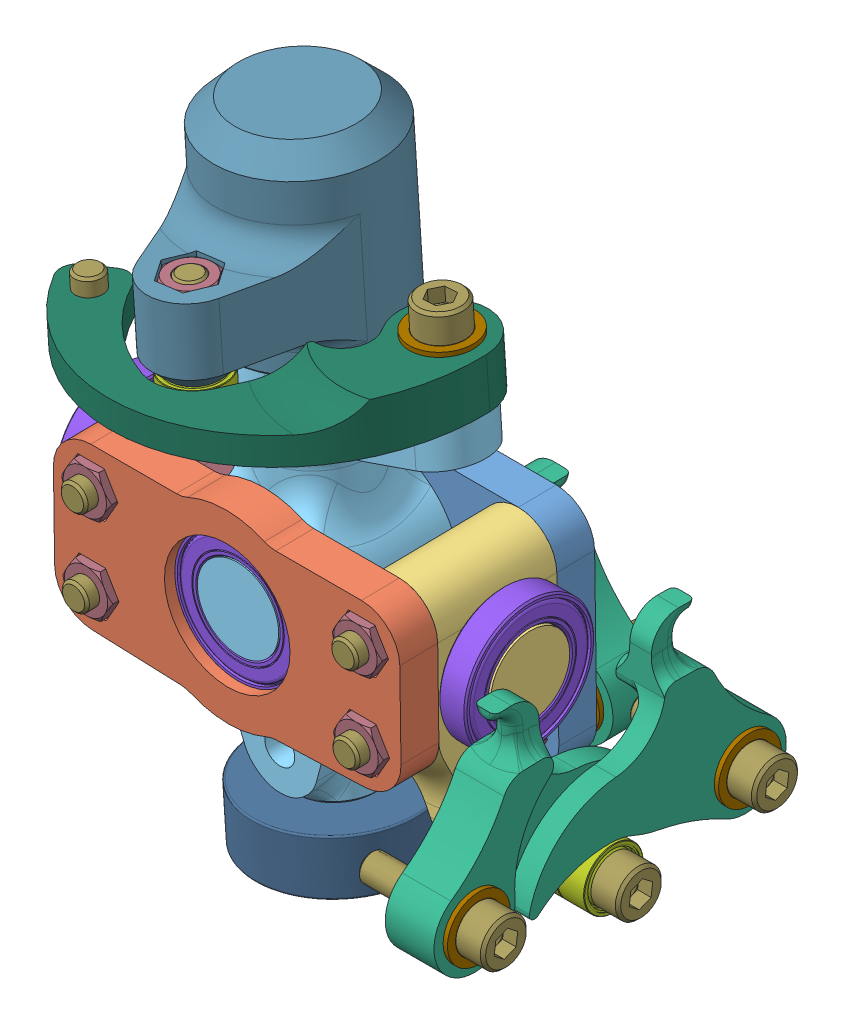
SolidWorks assembly Axis Assembly, configuration Default. Lengths in mm.
58 component instances, 15 part files, 133 mates.
Components (placement in the parent):
- gimbal_core_bearing_carrier_non_pot_side-1: gimbal_core_bearing_carrier_non_pot_side [Default] at (-18 0.2008 -14.4986) x (-1 0 0) z (0 0.013848 -0.999904) size (64 44 7.5)
- gimbal_core_bearing_carrier_pot_side-1: gimbal_core_bearing_carrier_pot_side [Default] at (-18 -0.2008 14.4986) x (1 0 0) z (0 -0.013848 0.999904) size (64 34.5 7)
- gimbal_core_non_pot_side-1: gimbal_core_non_pot_side [Default] x (0 0.013848 -0.999904) z (1 0 0) size (24.58 47 25)
- gimbal_core_pot_side-1: gimbal_core_pot_side [Default] at (-43 0 0) x (0 -0.013848 0.999904) z (-1 0 0) size (22 30 20)
- gimbal_lever_arm-1: gimbal_lever_arm [Default] at (-18 0 0) x (0.998482 0.055066 0.000763) z (0 0.013848 -0.999904) size (57.72 104.81 36)
- gimbal_cam-1: gimbal_cam [Default] at (25.5 -20.2447 24.8023) x (0 0.02979 -0.999556) z (1 0 0) size (47.46 36.5 9.63)
- gimbal_cam-2: gimbal_cam [Default] at (34.6 -19.7534 -25.1953) x (0 0.010459 0.999945) z (-1 0 0) size (47.46 36.5 9.63)
- gimbal_cam-3: gimbal_cam [Default] at (7 -19.7142 -20.775) x (-0.999486 0.032062 0.000444) z (0 0.013848 -0.999904) size (47.46 36.5 9.63)
- gimbal_cam-4: gimbal_cam [Default] at (-43 -19.5882 -29.8741) x (0.999746 0.022514 0.000312) z (0 -0.013848 0.999904) size (47.46 36.5 9.63)
- 685 Bearing-1: 685 Bearing [Default] at (-16.6232 -24.5775 -27.943) x (-0.212055 -0.977164 -0.013533) z (0 -0.013848 0.999904) size (11 11 5)
- 685 Bearing-2: 685 Bearing [Default] at (-16.6232 -24.6481 -22.8435) x (0.074604 0.997118 0.013809) z (0 -0.013848 0.999904) size (11 11 5)
- 685 Bearing-3: 685 Bearing [Default] at (27.5 -24.9976 -0.3462) x (0 0.011213 -0.999937) z (1 0 0) size (11 11 5)
- 685 Bearing-4: 685 Bearing [Default] at (32.6 -24.9976 -0.3462) x (0 0.989105 -0.147213) z (1 0 0) size (11 11 5)
- 6802 Bearing-1: 6802 Bearing [Default] at (-53.5 0 0) x (1 0 0) z (0 0.010217 0.999948) size (5 24 24)
- 6802 Bearing-2: 6802 Bearing [Default] at (17.5 0 0) x (1 0 0) z (0 -0.042847 0.999082) size (5 24 24)
- 6802 Bearing-3: 6802 Bearing [Default] at (-18 0.1869 -13.4987) x (0 -0.013848 0.999904) z (-0.979067 0.203518 0.002819) size (5 24 24)
- 6802 Bearing-4: 6802 Bearing [Default] at (-18 -0.1869 13.4987) x (0 0.013848 -0.999904) z (0.872831 -0.487976 -0.006758) size (5 24 24)
- MF105 Bearing-1: MF105 Bearing [Default] at (-43 -19.6048 -28.6742) x (1 0 0) z (0 -0.013848 0.999904) size (11.6 11.6 4)
- MF105 Bearing-2: MF105 Bearing [Default] at (-43 -19.6962 -22.0749) x (-0.910921 -0.412542 -0.005713) z (0 0.013848 -0.999904) size (11.6 11.6 4)
- MF105 Bearing-3: MF105 Bearing [Default] at (7 -19.6062 -28.5742) x (0.979695 0.200475 0.002776) z (0 -0.013848 0.999904) size (11.6 11.6 4)
- MF105 Bearing-4: MF105 Bearing [Default] at (7 -19.6976 -21.9749) x (-0.975001 0.222177 0.003077) z (0 0.013848 -0.999904) size (11.6 11.6 4)
- MF105 Bearing-5: MF105 Bearing [Default] at (33.3 -20.2447 24.8023) x (0 0.010217 0.999948) z (-1 0 0) size (11.6 11.6 4)
- MF105 Bearing-6: MF105 Bearing [Default] at (26.7 -20.2447 24.8023) x (0 -0.010217 -0.999948) z (1 0 0) size (11.6 11.6 4)
- MF105 Bearing-7: MF105 Bearing [Default] at (26.8 -19.7534 -25.1953) x (0 -0.010217 -0.999948) z (1 0 0) size (11.6 11.6 4)
- MF105 Bearing-8: MF105 Bearing [Default] at (33.4 -19.7534 -25.1953) x (0 0.010217 0.999948) z (-1 0 0) size (11.6 11.6 4)
- Magnetic Core-1: Magnetic Core [Default] at (-15.5873 -43.7393 -0.6058) x (0.998283 0.054779 0.020723) z (-0.019933 -0.014945 0.99969) size (30 10 30)
- flat washer narrow_am-2: flat washer narrow_am [B18.22M - Plain washer, 5 mm, narrow] at (-15.5873 -43.7393 -0.6058) x (-0.055071 0.998387 0.013827) z (0.032023 -0.012075 0.999414) size (1.4 11 11)
- socket head cap screw_am-1: socket head cap screw_am [B18.3.1M - 5 x 0.8 x 16 Hex SHCS -- 16NHX] at (-15.2349 -50.129 -0.6943) x (-0.055071 0.998387 0.013827) z (0.03273 -0.012036 0.999392) size (21 8.5 8.5)
- socket head cap screw_am-2: socket head cap screw_am [B18.3.1M - 5 x 0.8 x 35 Hex SHCS -- 22NHX] at (-43 8.2554 -18.3874) x (0 -0.013848 0.999904) z (-0.998547 -0.053881 -0.000746) size (40 8.5 8.5)
- socket head cap screw_am-3: socket head cap screw_am [B18.3.1M - 5 x 0.8 x 35 Hex SHCS -- 22NHX] at (-43 -7.743 -18.609) x (0 -0.013848 0.999904) z (-0.998547 -0.053881 -0.000746) size (40 8.5 8.5)
- socket head cap screw_am-4: socket head cap screw_am [B18.3.1M - 5 x 0.8 x 35 Hex SHCS -- 22NHX] at (7 8.2554 -18.3874) x (0 -0.013848 0.999904) z (-0.998547 -0.053881 -0.000746) size (40 8.5 8.5)
- socket head cap screw_am-5: socket head cap screw_am [B18.3.1M - 5 x 0.8 x 35 Hex SHCS -- 22NHX] at (7 -7.743 -18.609) x (0 -0.013848 0.999904) z (-0.998547 -0.053881 -0.000746) size (40 8.5 8.5)
- socket head cap screw_am-6: socket head cap screw_am [B18.3.1M - 5 x 0.8 x 20 Hex SHCS -- 20NHX] at (-43 -19.5079 -35.6736) x (0 -0.013848 0.999904) z (-0.998547 -0.053881 -0.000746) size (25 8.5 8.5)
- socket head cap screw_am-7: socket head cap screw_am [B18.3.1M - 5 x 0.8 x 20 Hex SHCS -- 20NHX] at (7 -19.5092 -35.5736) x (0 -0.013848 0.999904) z (-0.998547 -0.053881 -0.000746) size (25 8.5 8.5)
- socket head cap screw_am-8: socket head cap screw_am [B18.3.1M - 5 x 0.8 x 20 Hex SHCS -- 20NHX] at (40.4 -19.7534 -25.1953) x (-1 0 0) z (0 0.924225 0.381849) size (25 8.5 8.5)
- socket head cap screw_am-9: socket head cap screw_am [B18.3.1M - 5 x 0.8 x 20 Hex SHCS -- 20NHX] at (40.3 -20.2447 24.8023) x (-1 0 0) z (0 0.924225 0.381849) size (25 8.5 8.5)
- socket head cap screw_am-12: socket head cap screw_am [B18.3.1M - 5 x 0.8 x 25 Hex SHCS -- 25NHX] at (40.1 -24.9976 -0.3462) x (-1 0 0) z (0 0.924225 0.381849) size (30 8.5 8.5)
- socket head cap screw_am-13: socket head cap screw_am [B18.3.1M - 5 x 0.8 x 25 Hex SHCS -- 25NHX] at (-16.6232 -24.4736 -35.4423) x (0 -0.013848 0.999904) z (-0.998636 -0.052207 -0.000723) size (30 8.5 8.5)
- hex nut style 1_am-1: hex nut style 1_am [B18.2.4.1M - Hex nut, Style 1,  M5 x 0.8 --D-N] at (7 7.7334 19.3089) x (0.866025 -0.499952 -0.006924) z (0 -0.013848 0.999904) size (8 9.24 4.7)
- hex nut style 1_am-2: hex nut style 1_am [B18.2.4.1M - Hex nut, Style 1,  M5 x 0.8 --D-N] at (7 -8.2651 19.0874) x (0.866025 -0.499952 -0.006924) z (0 -0.013848 0.999904) size (8 9.24 4.7)
- hex nut style 1_am-3: hex nut style 1_am [B18.2.4.1M - Hex nut, Style 1,  M5 x 0.8 --D-N] at (-43 7.7334 19.3089) x (0.866025 -0.499952 -0.006924) z (0 -0.013848 0.999904) size (8 9.24 4.7)
- hex nut style 1_am-4: hex nut style 1_am [B18.2.4.1M - Hex nut, Style 1,  M5 x 0.8 --D-N] at (-43 -8.2651 19.0874) x (0.866025 -0.499952 -0.006924) z (0 -0.013848 0.999904) size (8 9.24 4.7)
- hex nut style 1_am-5: hex nut style 1_am [B18.2.4.1M - Hex nut, Style 1,  M5 x 0.8 --D-N] at (-43 -19.8624 -10.076) x (0.866025 -0.499952 -0.006924) z (0 -0.013848 0.999904) size (8 9.24 4.7)
- hex nut style 1_am-6: hex nut style 1_am [B18.2.4.1M - Hex nut, Style 1,  M5 x 0.8 --D-N] at (7 -19.8624 -10.076) x (0.866025 -0.499952 -0.006924) z (0 -0.013848 0.999904) size (8 9.24 4.7)
- hex nut style 1_am-7: hex nut style 1_am [B18.2.4.1M - Hex nut, Style 1,  M5 x 0.8 --D-N] at (10.3 -24.9976 -0.3462) x (0 -0.511945 0.859018) z (-1 0 0) size (8 9.24 4.7)
- 6802 Bearing-5: 6802 Bearing [Default] at (-20.2304 40.4347 0.56) x (-0.055071 0.998387 0.013827) z (0.998403 0.055236 -0.011824) size (5 24 24)
- 685 Bearing-5: 685 Bearing [Default] at (-21.497 63.3976 0.878) x (-0.802631 -0.036028 -0.595387) z (-0.055071 0.998387 0.013827) size (11 11 5)
- Grip attach-1: Grip attach [Default] at (-20.0927 37.9387 0.5254) x (-0.995007 -0.056029 0.082595) z (-0.083237 0.009209 -0.996487) size (31.31 35 45.5)
- 685 Bearing-6: 685 Bearing [Default] at (-18.2719 39.4241 23.4681) x (0.083237 -0.009209 0.996487) z (0.055071 -0.998387 -0.013827) size (11 11 5)
- socket head cap screw_am-14: socket head cap screw_am [B18.3.1M - 5 x 0.8 x 20 Hex SHCS -- 20NHX] at (-17.8589 31.9362 23.3644) x (-0.055071 0.998387 0.013827) z (0.280848 0.0022 0.95975) size (25 8.5 8.5)
- hex nut style 1_am-8: hex nut style 1_am [B18.2.4.1M - Hex nut, Style 1,  M5 x 0.8 --D-N] at (-18.9603 51.904 23.641) x (0.820083 0.053127 -0.569773) z (0.055071 -0.998387 -0.013827) size (8 9.24 4.7)
- gimbal_twist_cam-1: gimbal_twist_cam [Default] at (4.9134 38.5166 0.5334) x (-0.998296 -0.055323 0.018551) z (-0.019286 0.012782 -0.999732) size (61.45 9.74 43)
- MF105 Bearing-9: MF105 Bearing [Default] at (4.8473 39.7147 0.55) x (0.9981 0.054662 0.028435) z (-0.055071 0.998387 0.013827) size (11.6 11.6 4)
- MF105 Bearing-10: MF105 Bearing [Default] at (4.4838 46.3041 0.6413) x (-0.906258 -0.044167 -0.420412) z (0.055071 -0.998387 -0.013827) size (11.6 11.6 4)
- socket head cap screw_am-15: socket head cap screw_am [B18.3.1M - 5 x 0.8 x 20 Hex SHCS -- 20NHX] at (4.0983 53.2928 0.7381) x (0.055071 -0.998387 -0.013827) z (0.011142 -0.013233 0.99985) size (25 8.5 8.5)
- hex nut style 1_am-9: hex nut style 1_am [B18.2.4.1M - Hex nut, Style 1,  M5 x 0.8 --D-N] at (5.4256 29.2316 0.4048) x (0.998482 0.055066 0.000763) z (0.055071 -0.998387 -0.013827) size (8 9.24 4.7)
- socket head cap screw_am-16: socket head cap screw_am [B18.3.1M - 5 x 0.8 x 8 Hex SHCS -- 8NHX] at (-41.7595 30.6782 19.0099) x (-0.055071 0.998387 0.013827) z (0.153101 -0.005241 0.988197) size (13 8.5 8.5)
- socket head cap screw_am-17: socket head cap screw_am [B18.3.1M - 5 x 0.8 x 8 Hex SHCS -- 8NHX] at (-41.4755 40.4474 -12.6553) x (0.055071 -0.998387 -0.013827) z (0.189532 -0.003144 0.981869) size (13 8.5 8.5)
Mates (geometry in assembly coordinates):
- Coincident1: coincident aligned: plane of gimbal_core_non_pot_side-1 through (0 0 0) normal (1 0 0)
- Concentric11: concentric anti-aligned: cylinder of gimbal_core_non_pot_side-1 through (20 0 0) axis (-1 0 0) radius 7.3
- Coincident2: coincident anti-aligned: plane of gimbal_core_bearing_carrier_non_pot_side-1 through (-43 -19.8458 -11.2759) normal (0 -0.013848 0.999904); plane of gimbal_core_non_pot_side-1 through (14 -14.8462 -11.2067) normal (0 0.013848 -0.999904)
- Concentric12: concentric anti-aligned: cylinder of gimbal_core_bearing_carrier_non_pot_side-1 through (7 8.1516 -10.8882) axis (0 0.013848 -0.999904) radius 2.75; cylinder of gimbal_core_non_pot_side-1 through (7 7.9992 0.1108) axis (0 -0.013848 0.999904) radius 2.75
- Concentric13: concentric anti-aligned: cylinder of gimbal_core_bearing_carrier_non_pot_side-1 through (7 -7.8469 -11.1097) axis (0 0.013848 -0.999904) radius 2.75; cylinder of gimbal_core_non_pot_side-1 through (7 -7.9992 -0.1108) axis (0 -0.013848 0.999904) radius 2.75
- Coincident3: coincident anti-aligned: plane of gimbal_core_bearing_carrier_non_pot_side-1 through (-43 -19.8458 -11.2759) normal (0 -0.013848 0.999904); plane of gimbal_core_pot_side-1 through (-43 8.1516 -10.8882) normal (0 0.013848 -0.999904)
- Concentric14: concentric aligned: cylinder of gimbal_core_bearing_carrier_non_pot_side-1 through (-43 8.1516 -10.8882) axis (0 0.013848 -0.999904) radius 2.75; cylinder of gimbal_core_pot_side-1 through (-43 7.8469 11.1097) axis (0 0.013848 -0.999904) radius 2.75
- Concentric15: concentric aligned: cylinder of gimbal_core_bearing_carrier_non_pot_side-1 through (-43 -7.8469 -11.1097) axis (0 0.013848 -0.999904) radius 2.75; cylinder of gimbal_core_pot_side-1 through (-43 -8.1516 10.8882) axis (0 0.013848 -0.999904) radius 2.75
- Concentric16: concentric aligned: cylinder of gimbal_core_bearing_carrier_pot_side-1 through (-43 7.75 18.1091) axis (0 0.013848 -0.999904) radius 2.75; cylinder of gimbal_core_pot_side-1 through (-43 7.8469 11.1097) axis (0 0.013848 -0.999904) radius 2.75
- Concentric17: concentric aligned: cylinder of gimbal_core_bearing_carrier_pot_side-1 through (-43 -8.2485 17.8875) axis (0 0.013848 -0.999904) radius 2.75; cylinder of gimbal_core_pot_side-1 through (-43 -8.1516 10.8882) axis (0 0.013848 -0.999904) radius 2.75
- Coincident4: coincident anti-aligned: plane of gimbal_core_bearing_carrier_pot_side-1 through (-43 -8.1516 10.8882) normal (0 0.013848 -0.999904); plane of gimbal_core_pot_side-1 through (-43 7.8469 11.1097) normal (0 -0.013848 0.999904)
- Concentric18: concentric aligned: cylinder of gimbal_core_bearing_carrier_non_pot_side-1 through (-18 0.223 -16.0985) axis (0 -0.013848 0.999904) radius 12.1; cylinder of gimbal_lever_arm-1 through (-18 0.2216 -15.9985) axis (0 -0.013848 0.999904) radius 7.5
- Width1: width anti-aligned: plane of gimbal_core_bearing_carrier_non_pot_side-1 through (-43 -19.8458 -11.2759) normal (0 -0.013848 0.999904); plane of gimbal_lever_arm-1 through (-43 -8.1516 10.8882) normal (0 0.013848 -0.999904); plane of gimbal_core_bearing_carrier_pot_side-1 through (-18 0.2216 -15.9985) normal (0 0.013848 -0.999904); plane of gimbal_lever_arm-1 through (-18 -0.2216 15.9985) normal (0 -0.013848 0.999904)
- Concentric19: concentric anti-aligned: cylinder of gimbal_cam-1 through (29.5 -20.2447 24.8023) axis (-1 0 0) radius 5.1
- Concentric20: concentric aligned: cylinder of gimbal_cam-2 through (30.6 -19.7534 -25.1953) axis (1 0 0) radius 5.1
- Concentric21: concentric anti-aligned: cylinder of gimbal_core_bearing_carrier_non_pot_side-1 through (7 -19.8458 -11.2759) axis (0 0.013848 -0.999904) radius 2.75; cylinder of gimbal_cam-3 through (7 -19.6588 -24.7746) axis (0 -0.013848 0.999904) radius 5.1
- Concentric22: concentric aligned: cylinder of gimbal_core_bearing_carrier_non_pot_side-1 through (-43 -19.8458 -11.2759) axis (0 0.013848 -0.999904) radius 2.75; cylinder of gimbal_cam-4 through (-43 -19.6436 -25.8745) axis (0 0.013848 -0.999904) radius 5.1
- Concentric23: concentric aligned: cylinder of gimbal_lever_arm-1 through (-16.6232 -25.1812 15.6528) axis (0 0.013848 -0.999904) radius 2.75; cylinder of 685 Bearing-2 through (-16.6232 -24.6481 -22.8435) axis (0 0.013848 -0.999904) radius 2.5
- Concentric24: concentric aligned: cylinder of gimbal_lever_arm-1 through (-16.6232 -25.1812 15.6528) axis (0 0.013848 -0.999904) radius 2.75; cylinder of 685 Bearing-1 through (-16.6232 -24.5775 -27.943) axis (0 0.013848 -0.999904) radius 2.5
- Coincident7: coincident anti-aligned: plane of gimbal_lever_arm-1 through (-16.6232 -24.6827 -20.3438) normal (0 0.013848 -0.999904); plane of 685 Bearing-2 through (-19.1163 -24.4962 -20.3412) normal (0 -0.013848 0.999904)
- Distance3: distance = 0.1 mm anti-aligned: plane of 685 Bearing-2 through (-19.1163 -24.427 -25.3407) normal (0 0.013848 -0.999904); plane of 685 Bearing-1 through (-14.1801 -25.1422 -25.4506) normal (0 -0.013848 0.999904)
- PathMate2: path: point of 685 Bearing-1; curve of gimbal_cam-4; curve of gimbal_cam-4
- PathMate3: path: point of 685 Bearing-2; curve of gimbal_cam-3; curve of gimbal_cam-3
- LimitAngle1: limit planar angle = 0.055099 rad anti-aligned: plane of gimbal_lever_arm-1 through (-18 0 0) normal (0.998482 0.055066 0.000763); plane of gimbal_core_bearing_carrier_non_pot_side-1 through (-18 0.2008 -14.4986) normal (-1 0 0)
- LimitAngle2: limit planar angle = 0.013849 rad anti-aligned: plane of gimbal_core_non_pot_side-1 through (0 0 0) normal (0 0.013848 -0.999904)
- Concentric25: concentric anti-aligned: cylinder of gimbal_core_non_pot_side-1 through (0 -24.9976 -0.3462) axis (1 0 0) radius 2.75; cylinder of 685 Bearing-4 through (32.6 -24.9976 -0.3462) axis (-1 0 0) radius 2.5
- Concentric26: concentric anti-aligned: cylinder of gimbal_core_non_pot_side-1 through (0 -24.9976 -0.3462) axis (1 0 0) radius 2.75; cylinder of 685 Bearing-3 through (27.5 -24.9976 -0.3462) axis (-1 0 0) radius 2.5
- Coincident10: coincident anti-aligned: plane of gimbal_core_non_pot_side-1 through (25 -29.4972 -0.4085) normal (1 0 0); plane of 685 Bearing-3 through (25 -22.4978 -0.3182) normal (-1 0 0)
- Distance4: distance = 0.1 mm anti-aligned: plane of 685 Bearing-3 through (30 -22.4978 -0.3182) normal (1 0 0); plane of 685 Bearing-4 through (30.1 -24.6296 2.1266) normal (-1 0 0)
- PathMate5: path: unknown of 685 Bearing-3; edge_curve of ?
- PathMate6: path: unknown of 685 Bearing-4; edge_curve of ?
- Concentric27: concentric anti-aligned: cylinder of gimbal_lever_arm-1 through (-18 0.2216 -15.9985) axis (0 -0.013848 0.999904) radius 7.5; cylinder of 6802 Bearing-3 through (-18 0.1523 -10.9989) axis (0 0.013848 -0.999904) radius 7.5
- Coincident13: coincident anti-aligned: plane of gimbal_lever_arm-1 through (-18 0.1523 -10.9989) normal (0 0.013848 -0.999904); plane of 6802 Bearing-3 through (-18 0.1523 -10.9989) normal (0 -0.013848 0.999904)
- Coincident14: coincident anti-aligned: plane of gimbal_core_pot_side-1 through (-51 0 0) normal (-1 0 0); plane of 6802 Bearing-1 through (-51 0 0) normal (1 0 0)
- Concentric28: concentric anti-aligned: cylinder of gimbal_core_pot_side-1 through (-56 0 0) axis (1 0 0) radius 7.3; cylinder of 6802 Bearing-1 through (-51 0 0) axis (-1 0 0) radius 7.5
- Coincident15: coincident anti-aligned: plane of gimbal_core_non_pot_side-1 through (15 0 0) normal (1 0 0); plane of 6802 Bearing-2 through (15 0 0) normal (-1 0 0)
- Concentric29: concentric aligned: cylinder of gimbal_core_non_pot_side-1 through (20 0 0) axis (-1 0 0) radius 7.3; cylinder of 6802 Bearing-2 through (20 0 0) axis (-1 0 0) radius 7.5
- Concentric30: concentric anti-aligned: cylinder of gimbal_lever_arm-1 through (-18 -0.2216 15.9985) axis (0 0.013848 -0.999904) radius 7.5; cylinder of 6802 Bearing-4 through (-18 -0.1523 10.9989) axis (0 -0.013848 0.999904) radius 7.5
- Coincident16: coincident anti-aligned: plane of gimbal_lever_arm-1 through (-18 -0.1523 10.9989) normal (0 -0.013848 0.999904); plane of 6802 Bearing-4 through (-18 -0.1523 10.9989) normal (0 0.013848 -0.999904)
- Coincident17: coincident anti-aligned: plane of gimbal_cam-4 through (-64.5374 10.9826 -20.4499) normal (0 -0.013848 0.999904); plane of MF105 Bearing-2 through (-45.0629 -15.1586 -20.8119) normal (0 0.013848 -0.999904)
- Concentric31: concentric aligned: cylinder of gimbal_cam-4 through (-43 -19.6436 -25.8745) axis (0 0.013848 -0.999904) radius 5.1; cylinder of MF105 Bearing-2 through (-43 -19.6962 -22.0749) axis (0 0.013848 -0.999904) radius 2.5
- Coincident18: coincident anti-aligned: plane of gimbal_cam-4 through (-64.5374 11.1072 -29.449) normal (0 0.013848 -0.999904); plane of MF105 Bearing-1 through (-43 -14.5887 -29.8049) normal (0 -0.013848 0.999904)
- Concentric32: concentric anti-aligned: cylinder of gimbal_cam-4 through (-43 -19.6436 -25.8745) axis (0 0.013848 -0.999904) radius 5.1; cylinder of MF105 Bearing-1 through (-43 -19.6048 -28.6742) axis (0 -0.013848 0.999904) radius 5
- Concentric33: concentric aligned: cylinder of gimbal_cam-3 through (7 -19.6588 -24.7746) axis (0 -0.013848 0.999904) radius 5.1; cylinder of MF105 Bearing-3 through (7 -19.6062 -28.5742) axis (0 -0.013848 0.999904) radius 5
- Coincident19: coincident anti-aligned: plane of gimbal_cam-3 through (28.8297 10.8987 -29.3519) normal (0 0.013848 -0.999904); plane of MF105 Bearing-3 through (5.9975 -14.6916 -29.7063) normal (0 -0.013848 0.999904)
- Concentric34: concentric anti-aligned: cylinder of gimbal_cam-3 through (7 -19.6588 -24.7746) axis (0 -0.013848 0.999904) radius 5.1; cylinder of MF105 Bearing-4 through (7 -19.6976 -21.9749) axis (0 0.013848 -0.999904) radius 5
- Coincident20: coincident anti-aligned: plane of gimbal_cam-3 through (28.8297 10.7741 -20.3528) normal (0 -0.013848 0.999904); plane of MF105 Bearing-4 through (8.111 -14.8397 -20.7075) normal (0 0.013848 -0.999904)
- Coincident21: coincident anti-aligned: plane of gimbal_cam-2 through (25.6 11.2024 -46.361) normal (-1 0 0); plane of MF105 Bearing-7 through (25.6 -14.7537 -25.2464) normal (1 0 0)
- Concentric35: concentric aligned: cylinder of gimbal_cam-2 through (30.6 -19.7534 -25.1953) axis (1 0 0) radius 5.1; cylinder of MF105 Bearing-7 through (26.8 -19.7534 -25.1953) axis (1 0 0) radius 5
- Coincident22: coincident anti-aligned: plane of gimbal_cam-2 through (34.6 11.2024 -46.361) normal (1 0 0); plane of MF105 Bearing-8 through (34.6 -14.7537 -25.2464) normal (-1 0 0)
- Concentric36: concentric anti-aligned: cylinder of gimbal_cam-2 through (30.6 -19.7534 -25.1953) axis (1 0 0) radius 5.1; cylinder of MF105 Bearing-8 through (33.4 -19.7534 -25.1953) axis (-1 0 0) radius 2.5
- Coincident23: coincident anti-aligned: plane of gimbal_cam-1 through (25.5 10.2962 46.5625) normal (-1 0 0); plane of MF105 Bearing-6 through (25.5 -15.2449 24.7512) normal (1 0 0)
- Concentric37: concentric anti-aligned: cylinder of gimbal_cam-1 through (29.5 -20.2447 24.8023) axis (-1 0 0) radius 5.1; cylinder of MF105 Bearing-6 through (26.7 -20.2447 24.8023) axis (1 0 0) radius 5
- Coincident24: coincident anti-aligned: plane of gimbal_cam-1 through (34.5 10.2962 46.5625) normal (1 0 0); plane of MF105 Bearing-5 through (34.5 -15.2449 24.7512) normal (-1 0 0)
- Concentric38: concentric aligned: cylinder of gimbal_cam-1 through (29.5 -20.2447 24.8023) axis (-1 0 0) radius 5.1; cylinder of MF105 Bearing-5 through (33.3 -20.2447 24.8023) axis (-1 0 0) radius 2.5
- Concentric39: concentric aligned: cylinder of gimbal_lever_arm-1 through (-15.5873 -43.7393 -0.6058) axis (-0.055071 0.998387 0.013827) radius 5; cylinder of Magnetic Core-1 through (-15.5873 -43.7393 -0.6058) axis (-0.055071 0.998387 0.013827) radius 5
- Concentric41: concentric aligned: cylinder of gimbal_lever_arm-1 through (-16.6117 -25.1693 -0.3486) axis (0.055071 -0.998387 -0.013827) radius 2.75; cylinder of flat washer narrow_am-2 through (-13.664 -78.608 -1.0887) axis (0.055071 -0.998387 -0.013827) radius 2.89
- Coincident27: coincident anti-aligned: plane of gimbal_lever_arm-1 through (-15.5873 -43.7393 -0.6058) normal (0.055071 -0.998387 -0.013827); plane of flat washer narrow_am-2 through (-18.4715 -43.8997 -0.5153) normal (-0.055071 0.998387 0.013827)
- Concentric42: concentric aligned: cylinder of gimbal_lever_arm-1 through (-16.6117 -25.1693 -0.3486) axis (0.055071 -0.998387 -0.013827) radius 2.75; cylinder of socket head cap screw_am-1 through (-13.4864 -81.8278 -1.1333) axis (0.055071 -0.998387 -0.013827) radius 4.25
- Coincident28: coincident anti-aligned: plane of flat washer narrow_am-2 through (-20.9991 -45.4422 -0.4529) normal (0.055071 -0.998387 -0.013827); plane of socket head cap screw_am-1 through (-19.7515 -45.3729 -0.4891) normal (-0.055071 0.998387 0.013827)
- Concentric43: concentric aligned: cylinder of gimbal_core_bearing_carrier_non_pot_side-1 through (-43 8.1516 -10.8882) axis (0 0.013848 -0.999904) radius 2.75; cylinder of socket head cap screw_am-2 through (-43 8.6951 -50.1344) axis (0 0.013848 -0.999904) radius 4.25
- Coincident29: coincident anti-aligned: plane of gimbal_core_bearing_carrier_non_pot_side-1 through (-43 8.1862 -13.3879) normal (0 0.013848 -0.999904); plane of socket head cap screw_am-2 through (-43.229 12.4296 -13.3292) normal (0 -0.013848 0.999904)
- Concentric44: concentric aligned: cylinder of gimbal_core_bearing_carrier_non_pot_side-1 through (-43 -7.8469 -11.1097) axis (0 0.013848 -0.999904) radius 2.75; cylinder of socket head cap screw_am-3 through (-43 -7.3034 -50.356) axis (0 0.013848 -0.999904) radius 4.25
- Coincident30: coincident anti-aligned: plane of gimbal_core_bearing_carrier_non_pot_side-1 through (-43 -7.8123 -13.6095) normal (0 0.013848 -0.999904); plane of socket head cap screw_am-3 through (-43.229 -3.5689 -13.5507) normal (0 -0.013848 0.999904)
- Concentric45: concentric aligned: cylinder of gimbal_core_bearing_carrier_non_pot_side-1 through (7 8.1862 -13.3879) axis (0 0.013848 -0.999904) radius 4.75; cylinder of socket head cap screw_am-4 through (7 8.6951 -50.1344) axis (0 0.013848 -0.999904) radius 4.25
- Coincident31: coincident anti-aligned: plane of gimbal_core_bearing_carrier_non_pot_side-1 through (7 8.1862 -13.3879) normal (0 0.013848 -0.999904); plane of socket head cap screw_am-4 through (6.771 12.4296 -13.3292) normal (0 -0.013848 0.999904)
- Concentric46: concentric aligned: cylinder of gimbal_core_bearing_carrier_non_pot_side-1 through (7 -7.8123 -13.6095) axis (0 0.013848 -0.999904) radius 4.75; cylinder of socket head cap screw_am-5 through (7 -7.3034 -50.356) axis (0 0.013848 -0.999904) radius 4.25
- Coincident32: coincident anti-aligned: plane of gimbal_core_bearing_carrier_non_pot_side-1 through (7 -7.8123 -13.6095) normal (0 0.013848 -0.999904); plane of socket head cap screw_am-5 through (6.771 -3.5689 -13.5507) normal (0 -0.013848 0.999904)
- Concentric47: concentric anti-aligned: cylinder of MF105 Bearing-1 through (-43 -19.6325 -26.6744) axis (0 -0.013848 0.999904) radius 3.0055; cylinder of socket head cap screw_am-6 through (-43 -19.0682 -67.4205) axis (0 0.013848 -0.999904) radius 4.25
- Coincident33: coincident anti-aligned: plane of MF105 Bearing-1 through (-43 -17.0773 -30.6394) normal (0 0.013848 -0.999904); plane of socket head cap screw_am-6 through (-43.229 -15.3337 -30.6153) normal (0 -0.013848 0.999904)
- Concentric48: concentric anti-aligned: cylinder of MF105 Bearing-3 through (7 -19.6339 -26.5744) axis (0 -0.013848 0.999904) radius 3.1345; cylinder of socket head cap screw_am-7 through (7 -19.0696 -67.3205) axis (0 0.013848 -0.999904) radius 4.25
- Coincident34: coincident anti-aligned: plane of MF105 Bearing-3 through (6.4988 -17.1295 -30.5401) normal (0 0.013848 -0.999904); plane of socket head cap screw_am-7 through (6.771 -15.3351 -30.5153) normal (0 -0.013848 0.999904)
- Concentric49: concentric anti-aligned: cylinder of MF105 Bearing-8 through (33.4 -19.7534 -25.1953) axis (-1 0 0) radius 5.8; cylinder of socket head cap screw_am-8 through (72.15 -19.7534 -25.1953) axis (1 0 0) radius 4.25
- Coincident35: coincident anti-aligned: plane of MF105 Bearing-8 through (35.4 -17.2535 -25.2208) normal (1 0 0); plane of socket head cap screw_am-8 through (35.4 -21.3763 -21.2673) normal (-1 0 0)
- Concentric50: concentric anti-aligned: cylinder of MF105 Bearing-5 through (31.3 -20.2447 24.8023) axis (-1 0 0) radius 3.1345; cylinder of socket head cap screw_am-9 through (72.05 -20.2447 24.8023) axis (1 0 0) radius 4.25
- Coincident36: coincident anti-aligned: plane of MF105 Bearing-5 through (35.3 -17.7448 24.7768) normal (1 0 0); plane of socket head cap screw_am-9 through (35.3 -21.8675 28.7302) normal (-1 0 0)
- Concentric51: concentric anti-aligned: cone of 685 Bearing-1 through (-16.6232 -24.5442 -30.3428) axis (0 -0.013848 0.999904); cylinder of socket head cap screw_am-11 through (-17.8858 -28.4038 -64.4549) axis (0 -0.052212 -0.998636) radius 4.25
- Coincident37: coincident anti-aligned: plane of 685 Bearing-1 through (-14.1801 -25.0729 -30.4501) normal (0 0.013848 -0.999904); plane of socket head cap screw_am-11 through (-18.1077 -22.2466 -27.9766) normal (0 0.052212 0.998636)
- Concentric52: concentric anti-aligned: cylinder of 685 Bearing-4 through (32.6 -24.9976 -0.3462) axis (-1 0 0) radius 3.0853; cylinder of socket head cap screw_am-12 through (71.85 -24.9976 -0.3462) axis (1 0 0) radius 4.25
- Coincident38: coincident anti-aligned: plane of 685 Bearing-4 through (35.1 -24.6296 2.1266) normal (1 0 0); plane of socket head cap screw_am-12 through (35.1 -26.6205 3.5818) normal (-1 0 0)
- Concentric53: concentric aligned: cylinder of 685 Bearing-1 through (-16.6232 -24.5775 -27.943) axis (0 0.013848 -0.999904) radius 3.0853; cylinder of socket head cap screw_am-13 through (-16.6232 -24.0339 -67.1893) axis (0 0.013848 -0.999904) radius 4.25
- Coincident39: coincident anti-aligned: plane of 685 Bearing-1 through (-14.1801 -25.0729 -30.4501) normal (0 0.013848 -0.999904); plane of socket head cap screw_am-13 through (-16.8451 -20.299 -30.384) normal (0 -0.013848 0.999904)
- Concentric54: concentric anti-aligned: cylinder of gimbal_core_bearing_carrier_pot_side-1 through (7 7.75 18.1091) axis (0 0.013848 -0.999904) radius 2.75; cylinder of hex nut style 1_am-1 through (7 8.0801 -5.7262) axis (0 -0.013848 0.999904) radius 2.5
- Coincident40: coincident anti-aligned: plane of gimbal_core_bearing_carrier_pot_side-1 through (-18 -0.2008 14.4986) normal (0 -0.013848 0.999904); plane of hex nut style 1_am-1 through (9.3094 11.7981 14.6648) normal (0 0.013848 -0.999904)
- Concentric55: concentric anti-aligned: cylinder of gimbal_core_bearing_carrier_pot_side-1 through (7 -8.2485 17.8875) axis (0 0.013848 -0.999904) radius 2.75; cylinder of hex nut style 1_am-2 through (7 -7.9184 -5.9477) axis (0 -0.013848 0.999904) radius 2.5
- Coincident41: coincident anti-aligned: plane of gimbal_core_bearing_carrier_pot_side-1 through (-18 -0.2008 14.4986) normal (0 -0.013848 0.999904); plane of hex nut style 1_am-2 through (9.3094 -4.2004 14.4432) normal (0 0.013848 -0.999904)
- Concentric56: concentric anti-aligned: cylinder of gimbal_core_bearing_carrier_pot_side-1 through (-43 7.75 18.1091) axis (0 0.013848 -0.999904) radius 2.75; cylinder of hex nut style 1_am-3 through (-43 8.0801 -5.7262) axis (0 -0.013848 0.999904) radius 2.5
- Coincident42: coincident anti-aligned: plane of gimbal_core_bearing_carrier_pot_side-1 through (-18 -0.2008 14.4986) normal (0 -0.013848 0.999904); plane of hex nut style 1_am-3 through (-40.6906 11.7981 14.6648) normal (0 0.013848 -0.999904)
- Concentric57: concentric anti-aligned: cylinder of gimbal_core_bearing_carrier_pot_side-1 through (-43 -8.2485 17.8875) axis (0 0.013848 -0.999904) radius 2.75; cylinder of hex nut style 1_am-4 through (-43 -7.9184 -5.9477) axis (0 -0.013848 0.999904) radius 2.5
- Coincident43: coincident anti-aligned: plane of gimbal_core_bearing_carrier_pot_side-1 through (-18 -0.2008 14.4986) normal (0 -0.013848 0.999904); plane of hex nut style 1_am-4 through (-40.6906 -4.2004 14.4432) normal (0 0.013848 -0.999904)
- Concentric58: concentric anti-aligned: cylinder of gimbal_core_bearing_carrier_non_pot_side-1 through (-43 -19.8458 -11.2759) axis (0 0.013848 -0.999904) radius 2.75; cylinder of hex nut style 1_am-5 through (-43 -19.5157 -35.1111) axis (0 -0.013848 0.999904) radius 2.5
- Coincident44: coincident anti-aligned: plane of gimbal_core_bearing_carrier_non_pot_side-1 through (-18 0.2008 -14.4986) normal (0 -0.013848 0.999904); plane of hex nut style 1_am-5 through (-40.6906 -15.7977 -14.7202) normal (0 0.013848 -0.999904)
- Concentric59: concentric anti-aligned: cylinder of gimbal_core_bearing_carrier_non_pot_side-1 through (7 -19.8458 -11.2759) axis (0 0.013848 -0.999904) radius 2.75; cylinder of hex nut style 1_am-6 through (7 -19.5157 -35.1111) axis (0 -0.013848 0.999904) radius 2.5
- Coincident45: coincident anti-aligned: plane of gimbal_core_bearing_carrier_non_pot_side-1 through (-18 0.2008 -14.4986) normal (0 -0.013848 0.999904); plane of hex nut style 1_am-6 through (9.3094 -15.7977 -14.7202) normal (0 0.013848 -0.999904)
- Parallel1: parallel anti-aligned: plane of gimbal_core_bearing_carrier_pot_side-1 through (4.5463 -3.9504 14.4467) normal (0 -0.999904 -0.013848); plane of hex nut style 1_am-2 through (9.3094 -4.2004 14.4432) normal (0 0.999904 0.013848)
- Parallel2: parallel anti-aligned: plane of gimbal_core_bearing_carrier_pot_side-1 through (4.5463 12.048 14.6682) normal (0 -0.999904 -0.013848); plane of hex nut style 1_am-1 through (9.3094 11.7981 14.6648) normal (0 0.999904 0.013848)
- Parallel3: parallel anti-aligned: plane of gimbal_core_bearing_carrier_pot_side-1 through (-40.5463 12.048 14.6682) normal (0 -0.999904 -0.013848); plane of hex nut style 1_am-3 through (-40.6906 11.7981 14.6648) normal (0 0.999904 0.013848)
- Parallel4: parallel anti-aligned: plane of gimbal_core_bearing_carrier_pot_side-1 through (-40.5463 -3.9504 14.4467) normal (0 -0.999904 -0.013848); plane of hex nut style 1_am-4 through (-40.6906 -4.2004 14.4432) normal (0 0.999904 0.013848)
- Parallel5: parallel anti-aligned: plane of gimbal_core_bearing_carrier_non_pot_side-1 through (-40.5463 -15.5477 -14.7167) normal (0 -0.999904 -0.013848); plane of hex nut style 1_am-5 through (-40.6906 -15.7977 -14.7202) normal (0 0.999904 0.013848)
- Parallel6: parallel anti-aligned: plane of gimbal_core_bearing_carrier_non_pot_side-1 through (4.5463 -15.5477 -14.7167) normal (0 -0.999904 -0.013848); plane of hex nut style 1_am-6 through (9.3094 -15.7977 -14.7202) normal (0 0.999904 0.013848)
- Concentric60: concentric anti-aligned: cylinder of gimbal_core_non_pot_side-1 through (0 -24.9976 -0.3462) axis (1 0 0) radius 2.75; cylinder of hex nut style 1_am-7 through (35.3375 -24.9976 -0.3462) axis (-1 0 0) radius 2.5
- Coincident52: coincident anti-aligned: plane of gimbal_core_non_pot_side-1 through (15 0 0) normal (-1 0 0); plane of hex nut style 1_am-7 through (15 -21.03 2.0184) normal (1 0 0)
- Parallel7: parallel anti-aligned: plane of gimbal_core_non_pot_side-1 through (15 -29.2132 -2.8586) normal (0 0.999904 0.013848); plane of hex nut style 1_am-7 through (15 -28.9652 -2.7108) normal (0 -0.999904 -0.013848)
- Coincident53: coincident anti-aligned: plane of gimbal_lever_arm-1 through (-16.138 -33.7555 -0.4675) normal (0.055071 -0.998387 -0.013827); plane of Magnetic Core-1 through (-16.138 -33.7555 -0.4675) normal (-0.055071 0.998387 0.013827)
- Concentric61: concentric aligned: cylinder of gimbal_lever_arm-1 through (-15.5873 -43.7393 -0.6058) axis (0.055071 -0.998387 -0.013827) radius 7; cylinder of 6802 Bearing-5 through (-20.3681 42.9306 0.5946) axis (0.055071 -0.998387 -0.013827) radius 7.5
- Coincident54: coincident anti-aligned: plane of gimbal_lever_arm-1 through (-20.0927 38.0772 -9.4736) normal (-0.055071 0.998387 0.013827); plane of 6802 Bearing-5 through (-20.0927 37.9387 0.5254) normal (0.055071 -0.998387 -0.013827)
- Coincident55: coincident anti-aligned: plane of gimbal_lever_arm-1 through (-21.3594 60.9985 -6.1559) normal (-0.055071 0.998387 0.013827); plane of 685 Bearing-5 through (-22.8442 60.7919 2.8518) normal (0.055071 -0.998387 -0.013827)
- Concentric62: concentric anti-aligned: cylinder of gimbal_lever_arm-1 through (-20.3185 42.0321 0.5821) axis (-0.055071 0.998387 0.013827) radius 2.5; cylinder of 685 Bearing-5 through (-21.497 63.3976 0.878) axis (0.055071 -0.998387 -0.013827) radius 2.5
- Concentric63: concentric anti-aligned: cylinder of gimbal_lever_arm-1 through (-15.5873 -43.7393 -0.6058) axis (0.055071 -0.998387 -0.013827) radius 7; cylinder of Grip attach-1 through (-21.7449 67.8903 0.9402) axis (-0.055071 0.998387 0.013827) radius 7.5
- Coincident56: coincident aligned: plane of 6802 Bearing-5 through (-20.0927 37.9387 0.5254) normal (0.055071 -0.998387 -0.013827); plane of Grip attach-1 through (-20.0927 37.9387 0.5254) normal (0.055071 -0.998387 -0.013827)
- Concentric65: concentric aligned: cylinder of Grip attach-1 through (-18.4096 41.9201 23.5027) axis (-0.055071 0.998387 0.013827) radius 2.75; cylinder of 685 Bearing-6 through (-18.2719 39.4241 23.4681) axis (-0.055071 0.998387 0.013827) radius 2.5
- Concentric66: concentric anti-aligned: cylinder of 685 Bearing-6 through (-18.2719 39.4241 23.4681) axis (-0.055071 0.998387 0.013827) radius 3.0853; cylinder of socket head cap screw_am-14 through (-16.1103 0.2375 22.9254) axis (0.055071 -0.998387 -0.013827) radius 4.25
- Coincident60: coincident anti-aligned: plane of 685 Bearing-6 through (-20.6217 36.7881 23.6401) normal (0.055071 -0.998387 -0.013827); plane of socket head cap screw_am-14 through (-22.2064 36.687 24.6258) normal (-0.055071 0.998387 0.013827)
- Concentric67: concentric aligned: cylinder of socket head cap screw_am-14 through (-16.1103 0.2375 22.9254) axis (0.055071 -0.998387 -0.013827) radius 2.5; cylinder of hex nut style 1_am-8 through (-20.3391 76.9011 23.9872) axis (0.055071 -0.998387 -0.013827) radius 2.5
- Parallel8: parallel anti-aligned: plane of Grip attach-1 through (-21.9842 68.6999 28.3138) normal (-0.083237 0.009209 -0.996487); plane of hex nut style 1_am-8 through (-16.5883 56.6889 27.5012) normal (0.083237 -0.009209 0.996487)
- Coincident62: coincident anti-aligned: plane of Grip attach-1 through (-20.8747 52.1158 0.7218) normal (-0.055071 0.998387 0.013827); plane of hex nut style 1_am-8 through (-16.3295 51.9965 27.4362) normal (0.055071 -0.998387 -0.013827)
- Concentric68: concentric anti-aligned: cylinder of gimbal_twist_cam-1 through (4.4178 47.5021 0.6579) axis (0.055071 -0.998387 -0.013827) radius 5.1; cylinder of MF105 Bearing-9 through (4.8473 39.7147 0.55) axis (-0.055071 0.998387 0.013827) radius 5
- Coincident64: coincident anti-aligned: plane of gimbal_twist_cam-1 through (-20.044 37.1336 0.9972) normal (0.055071 -0.998387 -0.013827); plane of MF105 Bearing-9 through (5.0516 38.5935 -4.4641) normal (-0.055071 0.998387 0.013827)
- Concentric69: concentric anti-aligned: cylinder of gimbal_lever_arm-1 through (5.7334 23.6507 0.3275) axis (-0.055071 0.998387 0.013827) radius 2.5; cylinder of gimbal_twist_cam-1 through (4.4178 47.5021 0.6579) axis (0.055071 -0.998387 -0.013827) radius 5.1
- Coincident66: coincident anti-aligned: plane of gimbal_twist_cam-1 through (-20.5396 46.119 1.1216) normal (-0.055071 0.998387 0.013827); plane of MF105 Bearing-10 through (6.5134 47.6805 -3.8783) normal (0.055071 -0.998387 -0.013827)
- Concentric70: concentric aligned: cylinder of gimbal_twist_cam-1 through (4.4178 47.5021 0.6579) axis (0.055071 -0.998387 -0.013827) radius 5.1; cylinder of MF105 Bearing-10 through (4.4838 46.3041 0.6413) axis (0.055071 -0.998387 -0.013827) radius 5
- PathMate9: path: point of 685 Bearing-6; curve of gimbal_twist_cam-1; curve of gimbal_twist_cam-1
- Coincident67: coincident anti-aligned: plane of Grip attach-1 through (-18.4096 41.9201 23.5027) normal (0.055071 -0.998387 -0.013827); plane of 685 Bearing-6 through (-20.8971 41.78 23.7092) normal (-0.055071 0.998387 0.013827)
- Coincident68: coincident aligned: plane of Grip attach-1 through (-20.0927 37.9387 0.5254) normal (-0.995007 -0.056029 0.082595); plane of 685 Bearing-6 through (-18.2719 39.4241 23.4681) normal (-0.995007 -0.056029 0.082595)
- Concentric72: concentric anti-aligned: cylinder of MF105 Bearing-10 through (4.594 44.3073 0.6136) axis (0.055071 -0.998387 -0.013827) radius 3.0055; cylinder of socket head cap screw_am-15 through (2.3498 84.9915 1.1771) axis (-0.055071 0.998387 0.013827) radius 4.25
- Coincident70: coincident anti-aligned: plane of MF105 Bearing-10 through (5.4215 48.39 -1.5991) normal (-0.055071 0.998387 0.013827); plane of socket head cap screw_am-15 through (8.617 48.5355 0.6248) normal (0.055071 -0.998387 -0.013827)
- Concentric73: concentric anti-aligned: cylinder of gimbal_lever_arm-1 through (5.7334 23.6507 0.3275) axis (-0.055071 0.998387 0.013827) radius 2.5; cylinder of hex nut style 1_am-9 through (4.0467 54.2288 0.751) axis (0.055071 -0.998387 -0.013827) radius 2.5
- Coincident71: coincident anti-aligned: plane of gimbal_lever_arm-1 through (-19.7953 32.5474 0.4508) normal (0.055071 -0.998387 -0.013827); plane of hex nut style 1_am-9 through (5.1667 33.8601 5.0882) normal (-0.055071 0.998387 0.013827)
- Parallel9: parallel anti-aligned: plane of gimbal_lever_arm-1 through (10.0871 21.8539 2.7566) normal (-0.998482 -0.055066 -0.000763); plane of hex nut style 1_am-9 through (9.1607 34.1123 2.7821) normal (0.998482 0.055066 0.000763)
- Concentric4: concentric anti-aligned: cylinder of gimbal_twist_cam-1 through (-42.0348 35.6701 19.079) axis (-0.055071 0.998387 0.013827) radius 2.25; cylinder of socket head cap screw_am-16 through (-40.011 -1.0206 18.5709) axis (0.055071 -0.998387 -0.013827) radius 4.25
- Coincident9: coincident anti-aligned: plane of gimbal_twist_cam-1 through (-20.044 37.1336 0.9972) normal (0.055071 -0.998387 -0.013827); plane of socket head cap screw_am-16 through (-46.2282 35.4298 19.7274) normal (-0.055071 0.998387 0.013827)
- Concentric5: concentric aligned: cylinder of gimbal_lever_arm-1 through (-40.4209 21.3283 -12.9201) axis (-0.055071 0.998387 0.013827) radius 2.25; cylinder of socket head cap screw_am-17 through (-43.224 72.1462 -12.2163) axis (-0.055071 0.998387 0.013827) radius 4.25
- Coincident72: coincident anti-aligned: plane of gimbal_lever_arm-1 through (-20.0101 36.4411 0.5047) normal (-0.055071 0.998387 0.013827); plane of socket head cap screw_am-17 through (-37.0338 35.6964 -13.5279) normal (0.055071 -0.998387 -0.013827)
